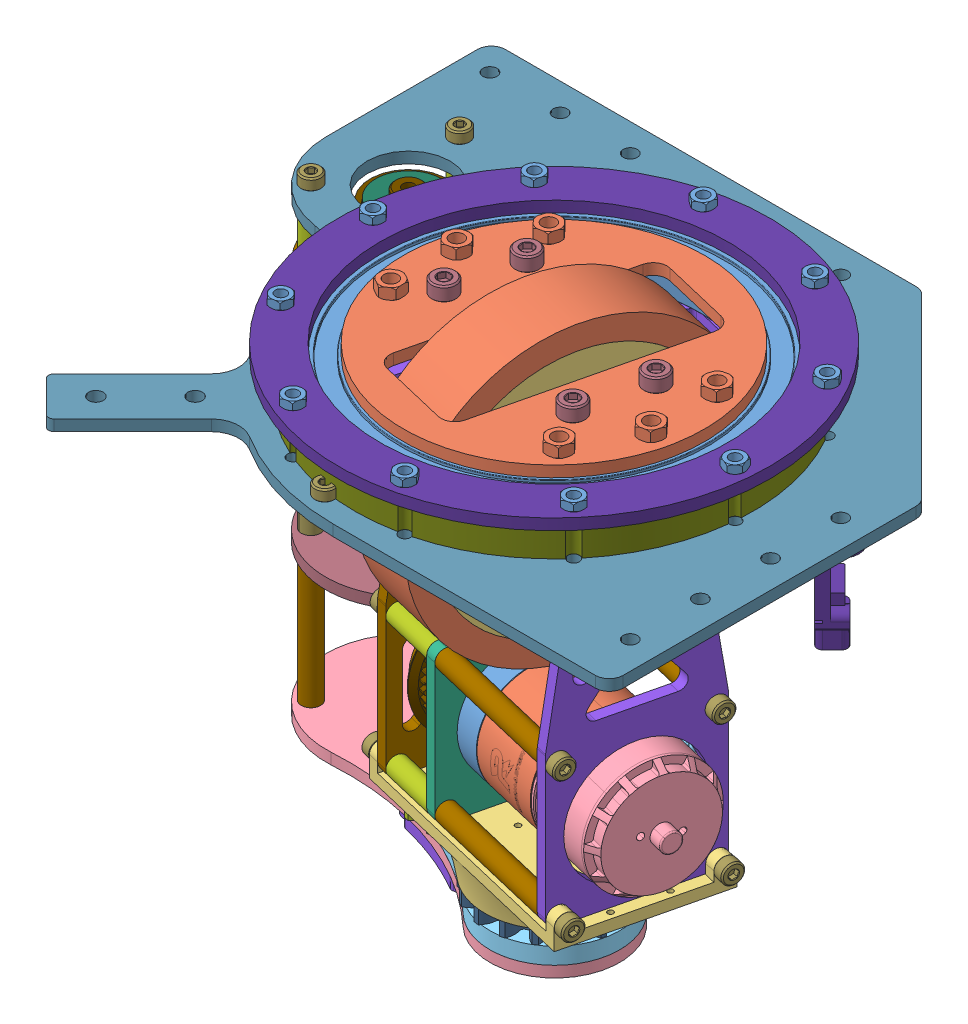
SolidWorks assembly 舵轮装配3508转向板R, configuration 默认. Lengths in mm. (continued)
Mates (geometry in assembly coordinates): (continued)
- 同心94: concentric aligned: cylinder of 舵轮上底板-1 through (14.1126 -87.8434 125.989) axis (0 -1 0) radius 2.6; cylinder of 舵轮转向同步轮 75齿-3 through (14.1126 -62.3434 125.989) axis (0 -1 0) radius 2.6
- 重合62: coincident aligned: plane of 舵轮转向同步轮 75齿-3 through (-20.4563 -97.8434 93.5041) normal (0 1 0); plane of 舵轮转向驱动同步轮15齿-1 through (-113.0601 -97.8434 53.3472) normal (0 1 0)
- 同心106: concentric anti-aligned: cylinder of 舵轮转向同步轮 75齿-3 through (-54.9022 -105.3434 60.7054) axis (0 -1 0) radius 4.5; cylinder of M5螺丝头-10 through (-54.9022 -110.3434 60.7054) axis (0 1 0) radius 4.35
- 同心107: concentric aligned: cylinder of M3508电机安装板-1 through (-58.4446 -100.8434 73.9963) axis (0.972741 0 0.231893) radius 2.6; cylinder of M5螺丝头-12 through (-63.3083 -100.8434 72.8368) axis (0.972741 0 0.231893) radius 4.35
- 重合64: coincident anti-aligned: plane of M3508电机安装板-1 through (-60.7636 -93.3434 83.7237) normal (-0.972741 0 -0.231893); plane of M5螺丝头-12 through (-58.4446 -100.8434 73.9963) normal (0.972741 0 0.231893)
- 重合65: coincident anti-aligned: plane of 舵轮转向同步轮 75齿-3 through (-66.6 -105.3434 82.3323) normal (0 -1 0); plane of M5螺丝头-11 through (-66.6 -105.3434 82.3323) normal (0 1 0)
- 同心108: concentric aligned: cylinder of 舵轮转向同步轮 75齿-3 through (-66.6 -105.3434 82.3323) axis (0 -1 0) radius 4.5; circle of M5螺丝头-11
- 同心109: concentric anti-aligned: cylinder of 舵轮转向同步轮 75齿-3 through (-65.9171 -105.3434 106.9107) axis (0 -1 0) radius 4.5; cylinder of M5螺丝头-13 through (-65.9171 -110.3434 106.9107) axis (0 1 0) radius 4.35
- 重合66: coincident anti-aligned: plane of 舵轮转向同步轮 75齿-3 through (-65.9171 -105.3434 106.9107) normal (0 -1 0); plane of M5螺丝头-13 through (-65.9171 -105.3434 106.9107) normal (0 1 0)
- 同心110: concentric aligned: cylinder of M3508电机安装板-1 through (-63.0825 -100.8434 93.4511) axis (0.972741 0 0.231893) radius 2.6; cylinder of M5螺丝头-14 through (-67.9462 -100.8434 92.2916) axis (0.972741 0 0.231893) radius 4.35
- 重合67: coincident anti-aligned: plane of M3508电机安装板-1 through (-60.7636 -93.3434 83.7237) normal (-0.972741 0 -0.231893); plane of M5螺丝头-14 through (-63.0825 -100.8434 93.4511) normal (0.972741 0 0.231893)
- 重合68: coincident anti-aligned: plane of 舵轮转向同步轮 75齿-3 through (-54.9022 -105.3434 60.7054) normal (0 -1 0); plane of M5螺丝头-10 through (-54.9022 -105.3434 60.7054) normal (0 1 0)
- 同心111: concentric anti-aligned: cylinder of 舵轮转向同步轮 75齿-3 through (25.1276 -105.3434 79.7838) axis (0 -1 0) radius 4.5; cylinder of M5螺丝头-7 through (25.1276 -110.3434 79.7838) axis (0 1 0) radius 4.35
- 同心112: concentric anti-aligned: cylinder of 舵轮转向同步轮 75齿-3 through (25.8104 -105.3434 104.3622) axis (0 -1 0) radius 4.5; cylinder of M5螺丝头-8 through (25.8104 -110.3434 104.3622) axis (0 1 0) radius 4.35
- 同心113: concentric anti-aligned: cylinder of 舵轮转向同步轮 75齿-3 through (14.1126 -105.3434 125.989) axis (0 -1 0) radius 4.5; cylinder of M5螺丝头-9 through (14.1126 -110.3434 125.989) axis (0 1 0) radius 4.35
- 重合69: coincident anti-aligned: plane of 舵轮转向同步轮 75齿-3 through (14.1126 -105.3434 125.989) normal (0 -1 0); plane of M5螺丝头-9 through (14.1126 -105.3434 125.989) normal (0 1 0)
- 重合70: coincident anti-aligned: plane of 舵轮转向同步轮 75齿-3 through (25.8104 -105.3434 104.3622) normal (0 -1 0); plane of M5螺丝头-8 through (25.8104 -105.3434 104.3622) normal (0 1 0)
- 重合71: coincident anti-aligned: plane of 舵轮转向同步轮 75齿-3 through (25.1276 -105.3434 79.7838) normal (0 -1 0); plane of M5螺丝头-7 through (25.1276 -105.3434 79.7838) normal (0 1 0)
- 同心114: concentric aligned: cylinder of HRB 61821薄圈轴承-1 through (-20.3948 -80.8434 93.3472) axis (0 -1 0) radius 65; cylinder of 舵轮大轴承定位环-1 through (-20.3948 -80.8434 93.3472) axis (0 -1 0) radius 72.1
- 同心116: concentric aligned: cylinder of 舵轮大轴承定位环-1 through (51.4309 -93.8434 99.6312) axis (0 1 0) radius 2.1; cylinder of 轴承压住-1 through (51.4309 -80.8434 99.6312) axis (0 1 0) radius 2.05
- 同心118: concentric aligned: cylinder of 舵轮大轴承定位环-1 through (34.0198 -93.8434 140.6491) axis (0 1 0) radius 2.1; circle of 轴承压住-1
- 重合77: coincident anti-aligned: plane of 舵轮大轴承定位环-1 through (-20.3948 -80.8434 93.3472) normal (0 1 0); plane of 轴承压住-1 through (-20.3948 -80.8434 93.3472) normal (0 -1 0)
- 重合80: coincident aligned: plane of M4螺丝头-17 through (7.7769 -101.8434 26.9788) normal (0 -1 0); plane of M4螺丝头-18 through (41.407 -101.8434 56.213) normal (0 -1 0)
- 重合81: coincident aligned: plane of M4螺丝头-16 through (-36.6138 -101.8434 23.0952) normal (0 -1 0); plane of M4螺丝头-17 through (7.7769 -101.8434 26.9788) normal (0 -1 0)
- 重合82: coincident aligned: plane of M4螺丝头-15 through (-74.8093 -101.8434 46.0454) normal (0 -1 0); plane of M4螺丝头-16 through (-36.6138 -101.8434 23.0952) normal (0 -1 0)
- 重合83: coincident aligned: plane of M4螺丝头-15 through (-74.8093 -101.8434 46.0454) normal (0 -1 0); plane of M4螺丝头-24 through (-92.2204 -101.8434 87.0633) normal (0 -1 0)
- 重合84: coincident aligned: plane of M4螺丝头-23 through (-82.1965 -101.8434 130.4815) normal (0 -1 0); plane of M4螺丝头-24 through (-92.2204 -101.8434 87.0633) normal (0 -1 0)
- 重合85: coincident aligned: plane of M4螺丝头-22 through (-48.5665 -101.8434 159.7156) normal (0 -1 0); plane of M4螺丝头-23 through (-82.1965 -101.8434 130.4815) normal (0 -1 0)
- 重合86: coincident aligned: plane of M4螺丝头-21 through (-4.1758 -101.8434 163.5993) normal (0 -1 0); plane of M4螺丝头-22 through (-48.5665 -101.8434 159.7156) normal (0 -1 0)
- 重合87: coincident aligned: plane of M4螺丝头-20 through (34.0198 -101.8434 140.6491) normal (0 -1 0); plane of M4螺丝头-21 through (-4.1758 -101.8434 163.5993) normal (0 -1 0)
- 重合88: coincident aligned: plane of M4螺丝头-19 through (51.4309 -101.8434 99.6312) normal (0 -1 0); plane of M4螺丝头-20 through (34.0198 -101.8434 140.6491) normal (0 -1 0)
- 同心131: concentric anti-aligned: cylinder of 轴承压住-1 through (41.407 -80.8434 56.213) axis (0 1 0) radius 2.05; cylinder of M4螺母-10 through (41.407 -73.8434 56.213) axis (0 -1 0) radius 2
- 同心132: concentric anti-aligned: cylinder of 轴承压住-1 through (51.4309 -80.8434 99.6312) axis (0 1 0) radius 2.05; cylinder of M4螺母-1 through (51.4309 -73.8434 99.6312) axis (0 -1 0) radius 2
- 同心133: concentric anti-aligned: cylinder of 轴承压住-1 through (34.0198 -80.8434 140.6491) axis (0 1 0) radius 2.05; cylinder of M4螺母-11 through (34.0198 -73.8434 140.6491) axis (0 -1 0) radius 2
- 同心134: concentric anti-aligned: cylinder of 轴承压住-1 through (-4.1758 -80.8434 163.5993) axis (0 1 0) radius 2.05; cylinder of M4螺母-3 through (-4.1758 -73.8434 163.5993) axis (0 -1 0) radius 2
- 同心135: concentric anti-aligned: cylinder of 轴承压住-1 through (-48.5665 -80.8434 159.7156) axis (0 1 0) radius 2.05; cylinder of M4螺母-4 through (-48.5665 -73.8434 159.7156) axis (0 -1 0) radius 2
- 同心136: concentric anti-aligned: cylinder of 轴承压住-1 through (-82.1965 -80.8434 130.4815) axis (0 1 0) radius 2.05; cylinder of M4螺母-5 through (-82.1965 -73.8434 130.4815) axis (0 -1 0) radius 2
- 同心137: concentric anti-aligned: cylinder of 轴承压住-1 through (-92.2204 -80.8434 87.0633) axis (0 1 0) radius 2.05; cylinder of M4螺母-6 through (-92.2204 -73.8434 87.0633) axis (0 -1 0) radius 2
- 同心138: concentric anti-aligned: cylinder of 轴承压住-1 through (-74.8093 -80.8434 46.0454) axis (0 1 0) radius 2.05; cylinder of M4螺母-7 through (-74.8093 -73.8434 46.0454) axis (0 -1 0) radius 2
- 同心139: concentric anti-aligned: cylinder of 轴承压住-1 through (7.7769 -80.8434 26.9788) axis (0 1 0) radius 2.05; cylinder of M4螺母-9 through (7.7769 -73.8434 26.9788) axis (0 -1 0) radius 2
- 同心140: concentric anti-aligned: cylinder of 轴承压住-1 through (-36.6138 -80.8434 23.0952) axis (0 1 0) radius 2.05; cylinder of M4螺母-8 through (-36.6138 -73.8434 23.0952) axis (0 -1 0) radius 2
- 重合89: coincident anti-aligned: plane of 轴承压住-1 through (-20.3948 -76.8434 93.3472) normal (0 1 0); plane of M4螺母-10 through (41.407 -76.8434 56.213) normal (0 -1 0)
- 重合90: coincident aligned: plane of M4螺母-9 through (7.7769 -73.8434 26.9788) normal (0 1 0); plane of M4螺母-10 through (41.407 -73.8434 56.213) normal (0 1 0)
- 重合91: coincident aligned: plane of M4螺母-8 through (-36.6138 -73.8434 23.0952) normal (0 1 0); plane of M4螺母-9 through (7.7769 -73.8434 26.9788) normal (0 1 0)
- 重合92: coincident aligned: plane of M4螺母-7 through (-74.8093 -73.8434 46.0454) normal (0 1 0); plane of M4螺母-8 through (-36.6138 -73.8434 23.0952) normal (0 1 0)
- 重合93: coincident aligned: plane of M4螺母-6 through (-92.2204 -73.8434 87.0633) normal (0 1 0); plane of M4螺母-7 through (-74.8093 -73.8434 46.0454) normal (0 1 0)
- 重合94: coincident aligned: plane of M4螺母-5 through (-82.1965 -73.8434 130.4815) normal (0 1 0); plane of M4螺母-6 through (-92.2204 -73.8434 87.0633) normal (0 1 0)
- 重合95: coincident aligned: plane of M4螺母-4 through (-48.5665 -73.8434 159.7156) normal (0 1 0); plane of M4螺母-5 through (-82.1965 -73.8434 130.4815) normal (0 1 0)
- 重合96: coincident aligned: plane of M4螺母-3 through (-4.1758 -73.8434 163.5993) normal (0 1 0); plane of M4螺母-4 through (-48.5665 -73.8434 159.7156) normal (0 1 0)
- 重合97: coincident aligned: plane of M4螺母-3 through (-4.1758 -73.8434 163.5993) normal (0 1 0); plane of M4螺母-11 through (34.0198 -73.8434 140.6491) normal (0 1 0)
- 重合98: coincident aligned: plane of M4螺母-1 through (51.4309 -73.8434 99.6312) normal (0 1 0); plane of M4螺母-11 through (34.0198 -73.8434 140.6491) normal (0 1 0)
- 同心141: concentric aligned: cylinder of 舵轮底板-1 through (11.1997 -70.8434 88.0288) axis (0 -1 0) radius 2.6; cylinder of M5螺丝头-18 through (11.1997 -71.8434 88.0288) axis (0 -1 0) radius 4.35
- 同心142: concentric aligned: cylinder of 舵轮底板-1 through (5.4024 -70.8434 112.3474) axis (0 -1 0) radius 2.6; cylinder of M5螺丝头-17 through (5.4024 -71.8434 112.3474) axis (0 -1 0) radius 4.35
- 同心143: concentric aligned: cylinder of 舵轮底板-1 through (-50.083 19.1566 73.4196) axis (0 -1 0) radius 2.6; cylinder of M5螺丝头-15 through (-50.083 -71.8434 73.4196) axis (0 -1 0) radius 4.35
- 同心144: concentric aligned: cylinder of 舵轮底板-1 through (-55.8803 19.1566 97.7381) axis (0 -1 0) radius 2.6; cylinder of M5螺丝头-16 through (-55.8803 -71.8434 97.7381) axis (0 -1 0) radius 4.35
- 重合99: coincident anti-aligned: plane of 舵轮底板-1 through (-20.3948 -76.8434 93.3472) normal (0 1 0); circle of M5螺丝头-16
- 重合100: coincident aligned: plane of M5螺丝头-15 through (-50.083 -71.8434 73.4196) normal (0 1 0); plane of M5螺丝头-16 through (-55.8803 -71.8434 97.7381) normal (0 1 0)
- 重合101: coincident aligned: plane of M5螺丝头-16 through (-55.8803 -71.8434 97.7381) normal (0 1 0); plane of M5螺丝头-17 through (5.4024 -71.8434 112.3474) normal (0 1 0)
- 重合102: coincident aligned: plane of M5螺丝头-17 through (5.4024 -71.8434 112.3474) normal (0 1 0); plane of M5螺丝头-18 through (11.1997 -71.8434 88.0288) normal (0 1 0)
- 同心145: concentric aligned: cylinder of 螺纹M4_长度20铝柱-5 through (-118.8835 -97.8434 29.0349) axis (0 -1 0) radius 3.5; cylinder of M4螺丝头-26 through (-118.8835 -89.8434 29.0349) axis (0 -1 0) radius 3.6
- 同心146: concentric aligned: cylinder of 螺纹M4_长度20铝柱-6 through (-131.2035 -97.8434 70.5466) axis (0 -1 0) radius 3.5; cylinder of M4螺丝头-25 through (-131.2035 -89.8434 70.5466) axis (0 -1 0) radius 3.6
- 重合104: coincident aligned: plane of M4螺丝头-26 through (-118.8835 -89.8434 29.0349) normal (0 1 0); plane of M4螺丝头-27 through (-31.1775 -89.8434 165.6069) normal (0 1 0)
- 重合105: coincident aligned: plane of M4螺丝头-25 through (-131.2035 -89.8434 70.5466) normal (0 1 0); plane of M4螺丝头-26 through (-118.8835 -89.8434 29.0349) normal (0 1 0)
- 同心151: concentric aligned: cylinder of 舵轮底板-1 through (14.1126 -70.8434 125.989) axis (0 -1 0) radius 2.6; cylinder of M5螺母-1 through (14.1126 -72.8434 125.989) axis (0 -1 0) radius 2.5
- 同心152: concentric aligned: cylinder of 舵轮底板-1 through (25.8104 -70.8434 104.3622) axis (0 -1 0) radius 2.6; cylinder of M5螺母-2 through (25.8104 -72.8434 104.3622) axis (0 -1 0) radius 2.5
- 同心153: concentric aligned: cylinder of 舵轮底板-1 through (25.1276 -70.8434 79.7838) axis (0 -1 0) radius 2.6; cylinder of M5螺母-3 through (25.1276 -72.8434 79.7838) axis (0 -1 0) radius 2.5
- 同心154: concentric aligned: cylinder of 舵轮底板-1 through (-54.9022 -70.8434 60.7054) axis (0 -1 0) radius 2.6; cylinder of M5螺母-4 through (-54.9022 -72.8434 60.7054) axis (0 -1 0) radius 2.5
- 同心155: concentric aligned: cylinder of 舵轮底板-1 through (-66.6 -70.8434 82.3323) axis (0 -1 0) radius 2.6; cylinder of M5螺母-5 through (-66.6 -72.8434 82.3323) axis (0 -1 0) radius 2.5
- 同心156: concentric aligned: cylinder of 舵轮底板-1 through (-65.9171 -70.8434 106.9107) axis (0 -1 0) radius 2.6; cylinder of M5螺母-6 through (-65.9171 -72.8434 106.9107) axis (0 -1 0) radius 2.5
- 重合109: coincident anti-aligned: plane of 舵轮底板-1 through (-20.3948 -76.8434 93.3472) normal (0 1 0); plane of M5螺母-6 through (-65.9171 -76.8434 106.9107) normal (0 -1 0)
- 重合110: coincident aligned: plane of M5螺母-5 through (-66.6 -72.8434 82.3323) normal (0 1 0); plane of M5螺母-6 through (-65.9171 -72.8434 106.9107) normal (0 1 0)
- 重合111: coincident aligned: plane of M5螺母-4 through (-54.9022 -72.8434 60.7054) normal (0 1 0); plane of M5螺母-6 through (-65.9171 -72.8434 106.9107) normal (0 1 0)
- 重合112: coincident aligned: plane of M5螺母-3 through (25.1276 -72.8434 79.7838) normal (0 1 0); plane of M5螺母-4 through (-54.9022 -72.8434 60.7054) normal (0 1 0)
- 重合113: coincident aligned: plane of M5螺母-2 through (25.8104 -72.8434 104.3622) normal (0 1 0); plane of M5螺母-3 through (25.1276 -72.8434 79.7838) normal (0 1 0)
- 重合114: coincident aligned: plane of M5螺母-1 through (14.1126 -72.8434 125.989) normal (0 1 0); plane of M5螺母-2 through (25.8104 -72.8434 104.3622) normal (0 1 0)
- 同心168: concentric anti-aligned: cylinder of M3508电机安装板-1 through (-45.4707 -223.3254 62.6968) axis (-0.972741 0 -0.231893) radius 2.1; cylinder of 舵轮线引导和角度定位3D打印件-1 through (-59.0891 -223.3254 59.4503) axis (0.972741 0 0.231893) radius 2.1
- 同心169: concentric anti-aligned: cylinder of M3508电机安装板-1 through (-56.6016 -223.3254 109.3884) axis (-0.972741 0 -0.231893) radius 2.1; cylinder of 舵轮线引导和角度定位3D打印件-1 through (-70.2199 -223.3254 106.1419) axis (0.972741 0 0.231893) radius 2.1
- 重合125: coincident anti-aligned: plane of M3508电机安装板-1 through (-60.7636 -93.3434 83.7237) normal (-0.972741 0 -0.231893); plane of 舵轮线引导和角度定位3D打印件-1 through (-60.7636 -226.8254 83.7237) normal (0.972741 0 0.231893)
- 锁定2: lock: unknown of 舵轮转向驱动同步轮15齿-1; unknown of 舵轮转向同步带90齿5m-1
- 同心183: concentric aligned: cylinder of 理线和舵轮角度定位支撑-1 through (-38.9826 -232.3434 72.5564) axis (0 -1 0) radius 1.65; cylinder of 舵轮角度定位第二齿轮轴承锁定-1 through (-38.9826 -241.8434 72.5564) axis (0 -1 0) radius 1.6
- 同心184: concentric aligned: cylinder of 理线和舵轮角度定位支撑-1 through (-75.6038 -232.3434 56.8757) axis (0 -1 0) radius 1.65; cylinder of 舵轮角度定位第二齿轮轴承锁定-1 through (-75.6038 -241.8434 56.8757) axis (0 -1 0) radius 1.6
- 重合139: coincident anti-aligned: plane of 理线和舵轮角度定位支撑-1 through (-113.0601 -255.8434 53.3472) normal (0 1 0); plane of 舵轮角度定位第二齿轮轴承锁定-1 through (-61.8199 -255.8434 75.2877) normal (0 -1 0)
- 同心192: concentric aligned: cylinder of 舵轮线引导和角度定位3D打印件-1 through (28.7495 -223.3254 80.3903) axis (-0.972741 0 -0.231893) radius 2.1; cylinder of M4螺丝头-34 through (32.6404 -223.3254 81.3178) axis (-0.972741 0 -0.231893) radius 3.6
- 同心193: concentric aligned: cylinder of 舵轮线引导和角度定位3D打印件-1 through (17.6186 -223.3254 127.0818) axis (-0.972741 0 -0.231893) radius 2.1; cylinder of M4螺丝头-31 through (21.5096 -223.3254 128.0094) axis (-0.972741 0 -0.231893) radius 3.6
- 重合142: coincident aligned: plane of M4螺丝头-31 through (21.5096 -223.3254 128.0094) normal (0.972741 0 0.231893); plane of M4螺丝头-34 through (32.6404 -223.3254 81.3178) normal (0.972741 0 0.231893)
- 重合143: coincident anti-aligned: plane of 舵轮线引导和角度定位3D打印件-1 through (23.184 -226.8254 103.736) normal (0.972741 0 0.231893); plane of M4螺丝头-31 through (17.6186 -223.3254 127.0818) normal (-0.972741 0 -0.231893)
- 同心194: concentric aligned: cylinder of 舵轮线引导和角度定位3D打印件-1 through (-59.0891 -223.3254 59.4503) axis (0.972741 0 0.231893) radius 2.1; cylinder of M4螺丝头-32 through (-62.9801 -223.3254 58.5228) axis (0.972741 0 0.231893) radius 3.6
- 同心195: concentric aligned: cylinder of 舵轮线引导和角度定位3D打印件-1 through (-70.2199 -223.3254 106.1419) axis (0.972741 0 0.231893) radius 2.1; cylinder of M4螺丝头-33 through (-74.1109 -223.3254 105.2143) axis (0.972741 0 0.231893) radius 3.6
- 重合144: coincident anti-aligned: plane of 舵轮线引导和角度定位3D打印件-1 through (-64.6545 -226.8254 82.7961) normal (-0.972741 0 -0.231893); plane of M4螺丝头-32 through (-59.0891 -223.3254 59.4503) normal (0.972741 0 0.231893)
- 重合145: coincident aligned: plane of M4螺丝头-32 through (-62.9801 -223.3254 58.5228) normal (-0.972741 0 -0.231893); plane of M4螺丝头-33 through (-74.1109 -223.3254 105.2143) normal (-0.972741 0 -0.231893)
- 同心196: concentric aligned: cylinder of 理线和舵轮角度定位支撑-1 through (-89.0934 -259.8434 60.4602) axis (0 1 0) radius 2.1; cylinder of M4螺丝头-28 through (-89.0934 -263.8434 60.4602) axis (0 1 0) radius 3.6
- 重合146: coincident anti-aligned: plane of 理线和舵轮角度定位支撑-1 through (-113.0601 -259.8434 53.3472) normal (0 -1 0); plane of M4螺丝头-28 through (-89.0934 -259.8434 60.4602) normal (0 1 0)
- 同心197: concentric aligned: cylinder of 理线和舵轮角度定位支撑-1 through (-131.2035 -259.8434 70.5466) axis (0 1 0) radius 2.1; cylinder of M4螺丝头-30 through (-131.2035 -263.8434 70.5466) axis (0 1 0) radius 3.6
- 重合147: coincident aligned: plane of M4螺丝头-28 through (-89.0934 -263.8434 60.4602) normal (0 -1 0); plane of M4螺丝头-30 through (-131.2035 -263.8434 70.5466) normal (0 -1 0)
- 同心201: concentric aligned: cylinder of 理线和舵轮角度定位支撑-1 through (-84.6571 -232.3434 78.0189) axis (0 -1 0) radius 1.65; cylinder of 舵轮角度定位AS5600支撑-1 through (-84.6571 -259.8434 78.0189) axis (0 -1 0) radius 1.6
- 同心202: concentric aligned: cylinder of 理线和舵轮角度定位支撑-1 through (-75.6038 -232.3434 56.8757) axis (0 -1 0) radius 1.65; cylinder of 舵轮角度定位AS5600支撑-1 through (-75.6038 -259.8434 56.8757) axis (0 -1 0) radius 1.6
- 同心203: concentric anti-aligned: cylinder of 螺纹M4_长度20铝柱-5 through (-118.8835 -97.8434 29.0349) axis (0 -1 0) radius 2; cylinder of 舵轮转向电机安装件M3508版本-1 through (-118.8835 -121.8434 29.0349) axis (0 1 0) radius 2.1
- 重合150: coincident anti-aligned: plane of 螺纹M4_长度20铝柱-5 through (-118.8835 -117.8434 29.0349) normal (0 -1 0); plane of 舵轮转向电机安装件M3508版本-1 through (-113.0601 -117.8434 53.3472) normal (0 1 0)
- 同心206: concentric anti-aligned: cylinder of 螺纹M4_长度20铝柱-7 through (-89.0934 -97.8434 60.4602) axis (0 -1 0) radius 2; cylinder of 舵轮转向电机安装件M3508版本-1 through (-89.0934 -121.8434 60.4602) axis (0 1 0) radius 2.1
- 同心207: concentric aligned: cylinder of 舵轮转向电机安装件M3508版本-1 through (-100.3598 -134.8434 41.3077) axis (0 1 0) radius 2.1; cylinder of RoboMaster M3508直流无刷减速电-2/2_ASM-1/16_1-1 through (-100.3598 -121.8434 41.3077) axis (0 1 0) radius 1.65
- 同心208: concentric aligned: cylinder of 舵轮转向电机安装件M3508版本-1 through (-113.0601 -134.8434 53.3472) axis (0 1 0) radius 13.15; cylinder of RoboMaster M3508直流无刷减速电-2/2_ASM-1/16_1-1 through (-113.0601 -102.7242 53.3472) axis (0 1 0) radius 13
- 重合152: coincident anti-aligned: plane of 舵轮转向电机安装件M3508版本-1 through (-113.0601 -121.8434 53.3472) normal (0 -1 0); plane of RoboMaster M3508直流无刷减速电-2/2_ASM-1/16_1-1 through (-112.713 -121.8434 40.3519) normal (0 1 0)
- 重合154: coincident anti-aligned: plane of 螺纹M4_长度20铝柱-6 through (-131.2035 -117.8434 70.5466) normal (0 -1 0); plane of 舵轮转向电机安装件M3508版本-1 through (-113.0601 -117.8434 53.3472) normal (0 1 0)
- 同心210: concentric anti-aligned: cylinder of 舵轮线引导和角度定位3D打印件-1 through (-20.7352 -238.8254 93.2661) axis (0 -1 0) radius 15; cylinder of 舵轮转向齿轮拼接-1 through (-20.7352 -248.8254 93.2661) axis (0 1 0) radius 15
- 平行2: parallel anti-aligned: plane of 舵轮线引导和角度定位3D打印件-1 through (-3.9581 -238.8254 109.1362) normal (-0.285546 0 -0.958365); plane of 舵轮转向齿轮拼接-1 through (-26.0906 -238.8254 115.7306) normal (0.285546 0 0.958365)
- 重合159: coincident anti-aligned: plane of 舵轮线引导和角度定位3D打印件-1 through (-20.7352 -238.8254 93.2661) normal (0 -1 0); plane of 舵轮转向齿轮拼接-1 through (-20.7352 -238.8254 93.2661) normal (0 1 0)
- 同心211: concentric aligned: cylinder of 舵轮角度定位第二齿轮轴承锁定-1 through (-20.4526 -163.1046 93.0006) axis (0 -1 0) radius 13.6; cylinder of 27_20_4轴承-1 through (-20.4526 -251.8434 93.0006) axis (0 -1 0) radius 10
- 重合160: coincident anti-aligned: plane of 舵轮角度定位第二齿轮轴承锁定-1 through (-61.8199 -251.8434 75.2877) normal (0 -1 0); plane of 27_20_4轴承-1 through (-20.4526 -251.8434 93.0006) normal (0 1 0)
- 同心213: concentric anti-aligned: cylinder of 舵轮转向电机安装件M3508版本-1 through (-118.8835 -121.8434 29.0349) axis (0 1 0) radius 2.1; cylinder of 螺纹M4_长度80铝柱-4 through (-118.8835 -121.8434 29.0349) axis (0 -1 0) radius 3.5
- 同心214: concentric anti-aligned: cylinder of 舵轮转向电机安装件M3508版本-1 through (-131.2035 -121.8434 70.5466) axis (0 1 0) radius 2.1; cylinder of 螺纹M4_长度80铝柱-5 through (-131.2035 -121.8434 70.5466) axis (0 -1 0) radius 3.5
- 同心215: concentric anti-aligned: circle of 舵轮转向电机安装件M3508版本-1; cylinder of 螺纹M4_长度80铝柱-6 through (-89.0934 -121.8434 60.4602) axis (0 -1 0) radius 3.5
- 重合161: coincident anti-aligned: plane of 舵轮转向电机安装件M3508版本-1 through (-113.0601 -121.8434 53.3472) normal (0 -1 0); plane of 螺纹M4_长度80铝柱-5 through (-131.2035 -121.8434 70.5466) normal (0 1 0)
- 重合162: coincident anti-aligned: plane of 舵轮转向电机安装件M3508版本-1 through (-113.0601 -121.8434 53.3472) normal (0 -1 0); plane of 螺纹M4_长度80铝柱-4 through (-118.8835 -121.8434 29.0349) normal (0 1 0)
- 重合163: coincident anti-aligned: plane of 舵轮转向电机安装件M3508版本-1 through (-113.0601 -121.8434 53.3472) normal (0 -1 0); plane of 螺纹M4_长度80铝柱-6 through (-89.0934 -121.8434 60.4602) normal (0 1 0)
- 同心216: concentric anti-aligned: cylinder of 螺纹M4_长度80铝柱-5 through (-131.2035 -121.8434 70.5466) axis (0 -1 0) radius 2; cylinder of 舵轮转向电机安装件-3 through (-131.2035 -205.8434 70.5466) axis (0 1 0) radius 2.1
- 重合164: coincident anti-aligned: plane of 螺纹M4_长度80铝柱-5 through (-131.2035 -201.8434 70.5466) normal (0 -1 0); plane of 舵轮转向电机安装件-3 through (-113.0601 -201.8434 53.3472) normal (0 1 0)
- 同心217: concentric anti-aligned: cylinder of 螺纹M4_长度80铝柱-4 through (-118.8835 -121.8434 29.0349) axis (0 -1 0) radius 2; cylinder of 舵轮转向电机安装件-3 through (-118.8835 -205.8434 29.0349) axis (0 1 0) radius 2.1
- 同心218: concentric anti-aligned: cylinder of 舵轮转向电机安装件-3 through (-131.2035 -205.8434 70.5466) axis (0 1 0) radius 2.1; cylinder of 螺纹M4_长度50铝柱-8 through (-131.2035 -205.8434 70.5466) axis (0 -1 0) radius 3.5
- 同心219: concentric anti-aligned: cylinder of 舵轮转向电机安装件-3 through (-118.8835 -205.8434 29.0349) axis (0 1 0) radius 2.1; cylinder of 螺纹M4_长度50铝柱-9 through (-118.8835 -205.8434 29.0349) axis (0 -1 0) radius 3.5
- 同心220: concentric anti-aligned: cylinder of 舵轮转向电机安装件-3 through (-89.0934 -205.8434 60.4602) axis (0 1 0) radius 2.1; cylinder of 螺纹M4_长度50铝柱-10 through (-89.0934 -205.8434 60.4602) axis (0 -1 0) radius 3.5
- 重合165: coincident anti-aligned: plane of 舵轮转向电机安装件-3 through (-113.0601 -205.8434 53.3472) normal (0 -1 0); plane of 螺纹M4_长度50铝柱-10 through (-89.0934 -205.8434 60.4602) normal (0 1 0)
- 重合166: coincident anti-aligned: plane of 舵轮转向电机安装件-3 through (-113.0601 -205.8434 53.3472) normal (0 -1 0); plane of 螺纹M4_长度50铝柱-9 through (-118.8835 -205.8434 29.0349) normal (0 1 0)
- 重合167: coincident anti-aligned: plane of 舵轮转向电机安装件-3 through (-113.0601 -205.8434 53.3472) normal (0 -1 0); plane of 螺纹M4_长度50铝柱-8 through (-131.2035 -205.8434 70.5466) normal (0 1 0)
- 重合168: coincident anti-aligned: plane of 理线和舵轮角度定位支撑-1 through (-113.0601 -255.8434 53.3472) normal (0 1 0); plane of 螺纹M4_长度50铝柱-10 through (-89.0934 -255.8434 60.4602) normal (0 -1 0)
- 同心221: concentric anti-aligned: cylinder of 理线和舵轮角度定位支撑-1 through (-118.8835 -259.8434 29.0349) axis (0 1 0) radius 2.1; cylinder of 螺纹M4_长度50铝柱-9 through (-118.8835 -205.8434 29.0349) axis (0 -1 0) radius 2
- 同心222: concentric anti-aligned: cylinder of 理线和舵轮角度定位支撑-1 through (-131.2035 -259.8434 70.5466) axis (0 1 0) radius 2.1; cylinder of 螺纹M4_长度50铝柱-8 through (-131.2035 -205.8434 70.5466) axis (0 -1 0) radius 3.5
- 同心226: concentric aligned: cylinder of 舵轮大轴承定位环-1 through (-20.3948 -80.8434 93.3472) axis (0 -1 0) radius 72.1; cylinder of 舵轮直角安装架R-1 through (-20.3948 -93.8434 93.3472) axis (0 -1 0) radius 63
- 重合171: coincident anti-aligned: plane of M4螺丝头-17 through (7.7769 -97.8434 26.9788) normal (0 1 0); plane of 舵轮直角安装架R-1 through (-20.3948 -97.8434 93.3472) normal (0 -1 0)
- 同心227: concentric aligned: cylinder of M4螺丝头-17 through (7.7769 -101.8434 26.9788) axis (0 1 0) radius 3.6; cylinder of 舵轮直角安装架R-1 through (7.7769 -103.8434 26.9788) axis (0 1 0) radius 2.05
- 同心228: concentric aligned: cylinder of M4螺丝头-18 through (41.407 -101.8434 56.213) axis (0 1 0) radius 3.6; cylinder of 舵轮直角安装架R-1 through (41.407 -103.8434 56.213) axis (0 1 0) radius 2.05
- 同心229: concentric aligned: cylinder of 舵轮大轴承定位环-1 through (41.407 -93.8434 56.213) axis (0 1 0) radius 2.1; cylinder of 舵轮直角安装架R-1 through (41.407 -103.8434 56.213) axis (0 1 0) radius 2.05
- 同心230: concentric aligned: cylinder of 舵轮大轴承定位环-1 through (51.4309 -93.8434 99.6312) axis (0 1 0) radius 2.1; cylinder of M4螺丝头-19 through (51.4309 -101.8434 99.6312) axis (0 1 0) radius 3.6
- 同心231: concentric aligned: cylinder of 舵轮大轴承定位环-1 through (34.0198 -93.8434 140.6491) axis (0 1 0) radius 2.1; cylinder of M4螺丝头-20 through (34.0198 -101.8434 140.6491) axis (0 1 0) radius 3.6
- 同心232: concentric aligned: cylinder of 舵轮大轴承定位环-1 through (-4.1758 -93.8434 163.5993) axis (0 1 0) radius 2.1; cylinder of M4螺丝头-21 through (-4.1758 -101.8434 163.5993) axis (0 1 0) radius 3.6
- 同心233: concentric aligned: cylinder of 舵轮大轴承定位环-1 through (-48.5665 -93.8434 159.7156) axis (0 1 0) radius 2.1; cylinder of M4螺丝头-22 through (-48.5665 -101.8434 159.7156) axis (0 1 0) radius 3.6
- 同心234: concentric aligned: cylinder of 舵轮大轴承定位环-1 through (-82.1965 -93.8434 130.4815) axis (0 1 0) radius 2.1; cylinder of M4螺丝头-23 through (-82.1965 -101.8434 130.4815) axis (0 1 0) radius 3.6
- 同心235: concentric aligned: cylinder of 舵轮大轴承定位环-1 through (-92.2204 -93.8434 87.0633) axis (0 1 0) radius 2.1; cylinder of M4螺丝头-24 through (-92.2204 -101.8434 87.0633) axis (0 1 0) radius 3.6
- 同心236: concentric aligned: cylinder of 舵轮大轴承定位环-1 through (-74.8093 -93.8434 46.0454) axis (0 1 0) radius 2.1; cylinder of M4螺丝头-15 through (-74.8093 -101.8434 46.0454) axis (0 1 0) radius 3.6
- 同心237: concentric aligned: cylinder of 舵轮大轴承定位环-1 through (-36.6138 -93.8434 23.0952) axis (0 1 0) radius 2.1; cylinder of M4螺丝头-16 through (-36.6138 -101.8434 23.0952) axis (0 1 0) radius 3.6
- 重合172: coincident anti-aligned: plane of 舵轮大轴承定位环-1 through (-20.3948 -93.8434 93.3472) normal (0 -1 0); plane of 舵轮直角安装架R-1 through (-20.3948 -93.8434 93.3472) normal (0 1 0)
- 重合173: coincident anti-aligned: plane of HRB 61821薄圈轴承-1 through (-20.3948 -93.8434 93.3472) normal (0 -1 0); plane of 舵轮直角安装架R-1 through (-20.3948 -93.8434 93.3472) normal (0 1 0)
- 同心238: concentric anti-aligned: cylinder of 螺纹M4_长度20铝柱-5 through (-118.8835 -97.8434 29.0349) axis (0 -1 0) radius 3.5; cylinder of 舵轮直角安装架R-1 through (-118.8835 -103.8434 29.0349) axis (0 1 0) radius 2.1
- 同心239: concentric anti-aligned: cylinder of 舵轮转向驱动同步轮15齿-1 through (-113.0601 -93.3434 53.3472) axis (0 -1 0) radius 5.15; cylinder of RoboMaster M3508直流无刷减速电-2/2_ASM-1/17_1-1 through (-113.0601 -94.5434 53.3472) axis (0 1 0) radius 5
- 同心240: concentric anti-aligned: cylinder of 螺纹M4_长度20铝柱-6 through (-131.2035 -97.8434 70.5466) axis (0 -1 0) radius 3.5; cylinder of 舵轮直角安装架R-1 through (-131.2035 -103.8434 70.5466) axis (0 1 0) radius 2.1
- 同心241: concentric anti-aligned: cylinder of 螺纹M4_长度20铝柱-6 through (-131.2035 -97.8434 70.5466) axis (0 -1 0) radius 2; cylinder of 舵轮转向电机安装件M3508版本-1 through (-131.2035 -121.8434 70.5466) axis (0 1 0) radius 2.1
- 锁定3: lock: unknown of 舵轮转向同步轮 75齿-3; unknown of 舵轮转向同步带90齿5m-1
- 同心242: concentric aligned: cylinder of 舵轮角度定位AS5600支撑-1 through (-50.6603 -253.8434 70.8196) axis (0 -1 0) radius 1.35; cylinder of as5600安装架小-1 through (-50.6603 -261.8434 70.8196) axis (0 -1 0) radius 1.35
- 同心243: concentric aligned: cylinder of 舵轮角度定位AS5600支撑-1 through (-66.2879 -253.8434 64.1281) axis (0 -1 0) radius 1.35; cylinder of as5600安装架小-1 through (-66.2879 -261.8434 64.1281) axis (0 -1 0) radius 1.35
- 重合174: coincident anti-aligned: plane of 舵轮角度定位AS5600支撑-1 through (-61.8199 -261.8434 75.2877) normal (0 -1 0); plane of as5600安装架小-1 through (-61.8199 -261.8434 75.2877) normal (0 1 0)
- 重合175: coincident anti-aligned: plane of 舵轮角度定位第二齿轮轴承锁定-1 through (-61.8199 -249.8434 75.2877) normal (0 -1 0); plane of 6704zz轴承-1 through (-61.8199 -249.8434 75.2877) normal (0 1 0)
- 重合176: coincident anti-aligned: plane of 螺纹M4_长度20铝柱-5 through (-118.8835 -97.8434 29.0349) normal (0 1 0); plane of 舵轮直角安装架R-1 through (-20.3948 -97.8434 93.3472) normal (0 -1 0)
- 同心244: concentric anti-aligned: cylinder of 6704zz轴承-1 through (-61.8199 -249.8434 75.2877) axis (0 -1 0) radius 10; cylinder of 舵轮角度定位第二齿轮-1 through (-61.8199 -251.7434 75.2877) axis (0 1 0) radius 10
- 同心245: concentric anti-aligned: cylinder of 舵轮角度定位第二齿轮轴承锁定-1 through (-61.8199 -255.8434 75.2877) axis (0 1 0) radius 13.6; cylinder of 6704zz轴承-1 through (-61.8199 -249.8434 75.2877) axis (0 -1 0) radius 13.5
- 重合177: coincident anti-aligned: plane of 6704zz轴承-1 through (-61.8199 -249.8434 75.2877) normal (0 1 0); plane of 舵轮角度定位第二齿轮-1 through (-61.8199 -249.8434 75.2877) normal (0 -1 0)
- 重合178: coincident anti-aligned: plane of M4螺丝头-26 through (-118.8835 -93.8434 29.0349) normal (0 -1 0); plane of 舵轮直角安装架R-1 through (-20.3948 -93.8434 93.3472) normal (0 1 0)
- 重合179: coincident anti-aligned: plane of 螺纹M4_长度20铝柱-7 through (-89.0934 -97.8434 60.4602) normal (0 1 0); plane of 舵轮直角安装架R-1 through (-20.3948 -97.8434 93.3472) normal (0 -1 0)
- 同心246: concentric aligned: cylinder of 舵轮角度定位第二齿轮-1 through (-61.8199 -259.8434 75.2877) axis (0 1 0) radius 6; cylinder of 第二齿轮上固定-1 through (-61.8199 -253.8434 75.2877) axis (0 1 0) radius 6.05
- 重合181: coincident anti-aligned: plane of 6704zz轴承-1 through (-61.8199 -253.8434 75.2877) normal (0 -1 0); plane of 第二齿轮上固定-1 through (-61.8199 -253.8434 75.2877) normal (0 1 0)
- 同心248: concentric aligned: cylinder of 舵轮角度定位第二齿轮-1 through (-59.9262 -236.7434 81.5057) axis (0 -1 0) radius 1.65; cylinder of 第二齿轮上固定-1 through (-59.9262 -251.8434 81.5057) axis (0 -1 0) radius 1.65
- 重合182: coincident anti-aligned: plane of 理线和舵轮角度定位支撑-1 through (-113.0601 -259.8434 53.3472) normal (0 -1 0); plane of 舵轮角度定位AS5600支撑-1 through (-61.8199 -259.8434 75.2877) normal (0 1 0)
- 距离4: distance = 2 mm anti-aligned: plane of as5600安装架小-2 through (-61.8199 -265.8434 75.2877) normal (0 1 0); plane of as5600安装架小-1 through (-61.8199 -263.8434 75.2877) normal (0 -1 0)
- 同心249: concentric anti-aligned: cylinder of as5600安装架小-1 through (-57.3518 -261.8434 86.4473) axis (0 -1 0) radius 1.35; cylinder of as5600安装架小-2 through (-57.3518 -267.8434 86.4473) axis (0 1 0) radius 1.35
- 同心250: concentric anti-aligned: cylinder of 舵轮角度定位AS5600支撑-1 through (-50.6603 -253.8434 70.8196) axis (0 -1 0) radius 1.35; cylinder of as5600安装架小-2 through (-50.6603 -267.8434 70.8196) axis (0 1 0) radius 1.35
- 平行3: parallel anti-aligned: plane of 舵轮直角安装架R-1 through (-20.3948 -97.8434 -6.6528) normal (0 0 -1)
- 重合183: coincident anti-aligned: plane of 舵轮直角安装架R-1 through (-20.3948 -97.8434 93.3472) normal (0 -1 0); plane of 配电板支架R-1 through (31.5052 -97.8434 41.4472) normal (0 1 0)
- 同心251: concentric aligned: cylinder of 舵轮直角安装架R-1 through (-6.5948 -103.8434 3.3472) axis (0 1 0) radius 2.55; cylinder of 配电板支架R-1 through (-6.5948 -101.8434 3.3472) axis (0 1 0) radius 2.65
- 同心252: concentric aligned: cylinder of 舵轮直角安装架R-1 through (69.6052 -103.8434 79.5472) axis (0 1 0) radius 2.55; cylinder of 配电板支架R-1 through (69.6052 -101.8434 79.5472) axis (0 1 0) radius 2.65
- 同心253: concentric anti-aligned: cylinder of RoboMaster M3508直流无刷减速电-1/2_ASM-1/17_1-1 through (-60.0826 -199.3254 83.886) axis (-0.972741 0 -0.231893) radius 5; cylinder of 40齿3M同步轮-1 through (-74.1335 -199.3254 80.5364) axis (0.972741 0 0.231893) radius 5.15
- 同心255: concentric anti-aligned: cylinder of 22 8 7轴承-1 through (-15.0447 -115.8434 94.6227) axis (-0.972741 0 -0.231893) radius 4; cylinder of 舵轮用钢轴-1 through (-54.9271 -115.8434 85.1151) axis (0.972741 0 0.231893) radius 4
- 同心256: concentric aligned: cylinder of 16_8_5轴承-1 through (-27.5931 -115.8434 91.6312) axis (0.972741 0 0.231893) radius 8; cylinder of 包胶轮子装配-1/定制轮子铝合金部分-1 through (-104.5369 -115.8434 73.2885) axis (0.972741 0 0.231893) radius 8.1
- 同心257: concentric aligned: cylinder of 舵轮用钢轴-1 through (-54.9271 -115.8434 85.1151) axis (0.972741 0 0.231893) radius 4; cylinder of 包胶轮子装配-1/定制轮子铝合金部分-1 through (-104.5369 -115.8434 73.2885) axis (0.972741 0 0.231893) radius 8.1
- 重合187: coincident anti-aligned: plane of 22 8 7轴承-1 through (-10.181 -115.8434 95.7821) normal (-0.972741 0 -0.231893); plane of 包胶轮子装配-1/定制轮子铝合金部分-1 through (-10.181 -115.8434 95.7821) normal (0.972741 0 0.231893)
- 同心259: concentric aligned: cylinder of 22 8 7轴承-1 through (-10.181 -115.8434 95.7821) axis (0.972741 0 0.231893) radius 12.5; cylinder of 包胶轮子装配-1/定制轮子铝合金部分-1 through (-10.181 -115.8434 95.7821) axis (0.972741 0 0.231893) radius 12.6
- 重合188: coincident anti-aligned: plane of 16_8_5轴承-1 through (-31.484 -115.8434 90.7037) normal (0.972741 0 0.231893); plane of 包胶轮子装配-1/定制轮子铝合金部分-1 through (-31.484 -115.8434 90.7037) normal (-0.972741 0 -0.231893)
- 同心260: concentric anti-aligned: cylinder of 舵轮用钢轴-1 through (-54.9271 -115.8434 85.1151) axis (0.972741 0 0.231893) radius 4; cylinder of 包胶轮子同步轮-1 through (-7.517 -115.8434 96.4172) axis (-0.972741 0 -0.231893) radius 8.1
- 重合192: coincident anti-aligned: plane of 包胶轮子装配-1/定制轮子铝合金部分-1 through (-32.5541 -115.8434 90.4486) normal (-0.972741 0 -0.231893); plane of 包胶轮子同步轮-1 through (-52.2187 24.1318 172.9374) normal (0.972741 0 0.231893)
- 距离7: distance = 1 mm anti-aligned: plane of 包胶轮子同步轮-1 through (-45.975 -122.3307 77.7491) normal (-0.972741 0 -0.231893); plane of 舵轮侧面支撑B-1 through (-45.0325 -140.8434 69.4834) normal (0.972741 0 0.231893)
- 相切1: tangent aligned: plane of 舵轮用100齿3m同步带-1 through (-51.3465 -197.7877 107.5971) normal (-0.231276 0.072894 0.970154); cylinder of 包胶轮子同步轮-1 through (-46.6588 -115.8434 87.0861) axis (-0.972741 0 -0.231893) radius 15.0096
- 同心264: concentric aligned: cylinder of 舵轮用100齿3m同步带-1 through (-46.4677 -199.3254 87.1317) axis (0.972741 0 0.231893) radius 21.095; cylinder of 40齿3M同步轮-1 through (-50.3552 -199.3254 86.2049) axis (0.972741 0 0.231893) radius 18.7162
- 同心265: concentric anti-aligned: cylinder of 包胶轮子装配-1/定制轮子铝合金部分-1 through (-55.7765 -128.4183 105.9273) axis (0.972741 0 0.231893) radius 2.1; cylinder of 包胶轮子同步轮-1 through (-37.2944 -128.4183 110.3333) axis (-0.972741 0 -0.231893) radius 2.1
- 同心266: concentric aligned: cylinder of 舵轮用钢轴-1 through (-54.9271 -115.8434 85.1151) axis (0.972741 0 0.231893) radius 4; cylinder of 包胶轮子垫圈-1 through (-8.2355 -115.8434 96.2459) axis (0.972741 0 0.231893) radius 4.15
- 重合193: coincident anti-aligned: plane of 舵轮侧面支撑-1 through (-2.5662 -140.8434 115.5878) normal (-0.972741 0 -0.231893); plane of 包胶轮子垫圈-1 through (1.4919 -115.8434 98.5648) normal (0.972741 0 0.231893)
- 同心268: concentric aligned: cylinder of RoboMaster M3508直流无刷减速电-1/2_ASM-1/17_1-1 through (-51.2821 -199.1686 90.0929) axis (-0.231715 0.039213 0.971993) radius 1.25; cylinder of 40齿3M同步轮-1 through (-50.3442 -199.3273 86.1587) axis (-0.231715 0.039213 0.971993) radius 1.4841
